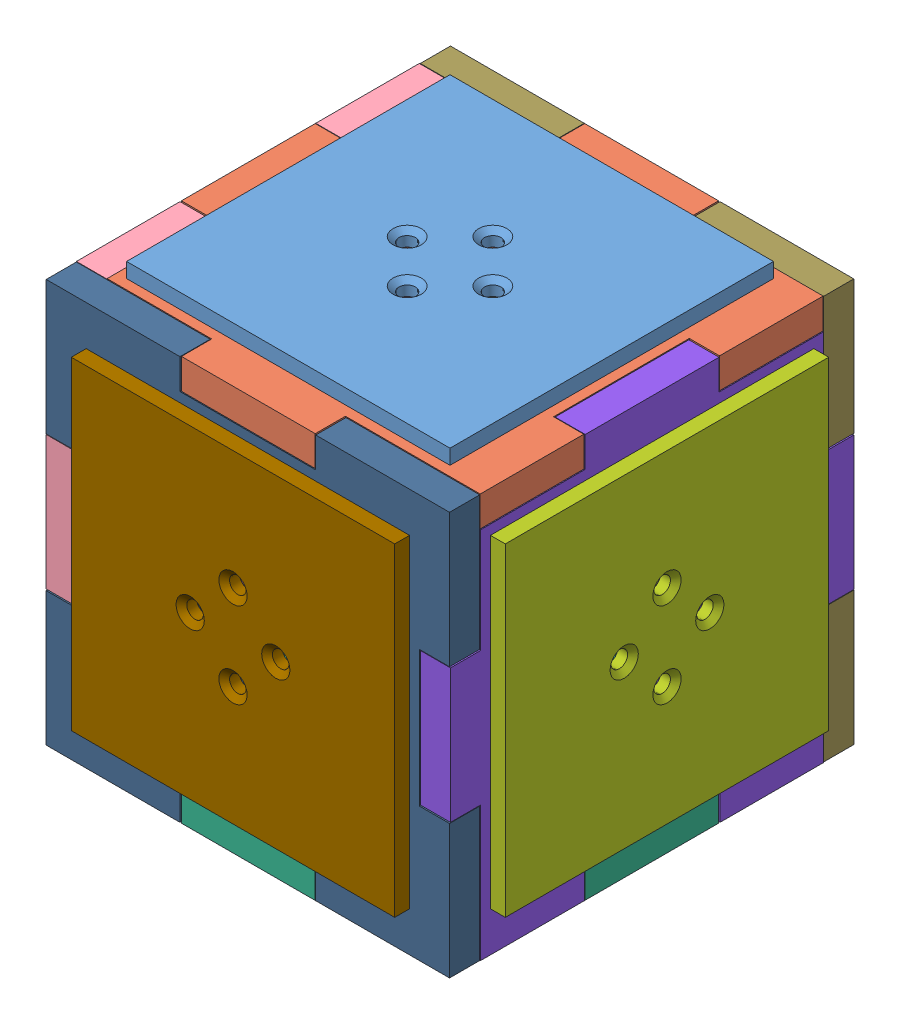
SolidWorks assembly cube_11, configuration cube11. Lengths in mm.
Overall size (46.52 46.39 46.35).
12 component instances, 12 part files, 6 mates.
Components (placement in the parent):
- panel_R^cube_11-13: panel_R^cube_11 [cube01] x (-1 0 0) z (0 0 1) size (28.76 1.62 34.54) (virtual)
- acrylic_R^cube_11-1: acrylic_R^cube_11 [A] at origin size (37.98 3.35 43.08) (virtual)
- panel_O^cube_11-8: panel_O^cube_11 [cube01] x (0 -1 0) z (0 0 1) size (28.03 1.76 34.54) (virtual)
- acrylic_O^cube_11-23: acrylic_O^cube_11 [A] x (0 1 0) z (0 0 1) size (37.56 3.45 43.08) (virtual)
- panel_Y^cube_11-9: panel_Y^cube_11 [cube01] at origin size (34.54 1.59 34.54) (virtual)
- acrylic_Y^cube_11-24: acrylic_Y^cube_11 [A] x (-1 0 0) z (0 0 1) size (43.08 3.23 43.08) (virtual)
- panel_G^cube_11-10: panel_G^cube_11 [cube01] x (0 1 0) z (0 0 1) size (34.54 1.59 34.54) (virtual)
- acrylic_G^cube_11-25: acrylic_G^cube_11 [A] x (0 -1 0) z (0 0 1) size (43.08 3.23 43.08) (virtual)
- panel_C^cube_11-11: panel_C^cube_11 [cube01] x (-1 0 0) z (0 -1 0) size (34.54 1.59 34.54) (virtual)
- acrylic_C^cube_11-26: acrylic_C^cube_11 [B] x (1 0 0) z (0 -1 0) size (43.08 3.23 43.08) (virtual)
- panel_B^cube_11-13: panel_B^cube_11 [cube01] x (-1 0 0) z (0 1 0) size (34.54 1.59 34.54) (virtual)
- acrylic_B^cube_11-27: acrylic_B^cube_11 [B] x (1 0 0) z (0 1 0) size (43.08 3.23 43.08) (virtual)
Mates (geometry in assembly coordinates):
- Coincident1: coincident aligned: plane of panel_R^cube_11-13 through (0 0 0) normal (0 0 1); plane of assembly through (0 0 0) normal (0 0 1)
- Coincident2: coincident anti-aligned: plane of panel_R^cube_11-13; plane of assembly through (0 0 0) normal (1 0 0)
- Coincident3: coincident anti-aligned: plane of panel_R^cube_11-13; plane of assembly through (0 0 0) normal (0 1 0)
- Coincident4: coincident aligned: plane of acrylic_R^cube_11-1 through (0 0 0) normal (0 0 1); plane of assembly through (0 0 0) normal (0 0 1)
- Coincident5: coincident aligned: plane of acrylic_R^cube_11-1 through (0 0 0) normal (1 0 0); plane of assembly through (0 0 0) normal (1 0 0)
- Coincident6: coincident aligned: plane of ? through (0 0 0) normal (0 1 0); plane of assembly through (0 0 0) normal (0 1 0)
